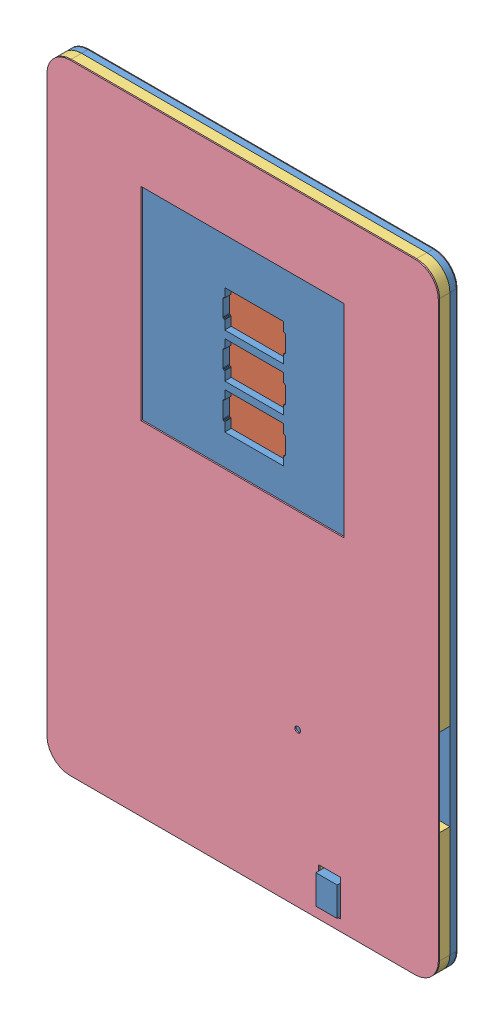
SolidWorks assembly 装配体1, configuration 默认. Lengths in mm.
Overall size (54 85.5 3.31).
4 component instances, 4 part files, 9 mates.
Components (placement in the parent):
- NFCard-1: NFCard [默认] at (-41.0066 8.8205 -0.55) size (54 85.5 3.31)
- 低-1: 低 [默认] at (-41.0066 8.8205 -1.5414) x (0 1 0) z (1 0 0) size (85.5 0.1 54)
- 顶1-1: 顶1 [默认] at (-41.0066 8.8205 -0.55) size (54 85.5 1.42)
- 顶2-1: 顶2 [默认] at (-41.0066 8.8205 0.87) size (54 85.5 0.18)
Mates (geometry in assembly coordinates):
- 重合1: coincident anti-aligned: plane of NFCard-1 through (-68.0066 -30.7495 -1.4414) normal (0 0 -1); plane of 低-1 through (-64.8266 -30.7495 -1.4414) normal (0 0 1)
- 重合2: coincident aligned: plane of NFCard-1 through (-68.0066 48.3905 -1.4414) normal (-1 0 0); plane of 低-1 through (-68.0066 -30.7495 -1.4414) normal (-1 0 0)
- 重合3: coincident aligned: plane of NFCard-1 through (-17.1866 51.5705 -1.4414) normal (0 1 0); plane of 低-1 through (-17.1866 51.5705 -1.4414) normal (0 1 0)
- 重合4: coincident anti-aligned: plane of NFCard-1 through (-68.0066 -30.7495 -0.55) normal (0 0 1); plane of 顶1-1 through (-17.1866 -30.7495 -0.55) normal (0 0 -1)
- 重合5: coincident aligned: plane of NFCard-1 through (-68.0066 48.3905 -1.4414) normal (-1 0 0); plane of 顶1-1 through (-68.0066 -30.7495 0.87) normal (-1 0 0)
- 重合6: coincident aligned: plane of NFCard-1 through (-64.8266 -33.9295 -1.4414) normal (0 -1 0); plane of 顶1-1 through (-64.8266 -33.9295 0.87) normal (0 -1 0)
- 重合7: coincident anti-aligned: plane of 顶1-1 through (-17.1866 -30.7495 0.87) normal (0 0 1); plane of 顶2-1 through (-64.8266 -30.7495 0.87) normal (0 0 -1)
- 重合8: coincident aligned: plane of 顶1-1 through (-68.0066 -30.7495 0.87) normal (-1 0 0); plane of 顶2-1 through (-68.0066 -30.7495 1.05) normal (-1 0 0)
- 重合9: coincident aligned: plane of 顶1-1 through (-64.8266 -33.9295 0.87) normal (0 -1 0); plane of 顶2-1 through (-64.8266 -33.9295 1.05) normal (0 -1 0)
